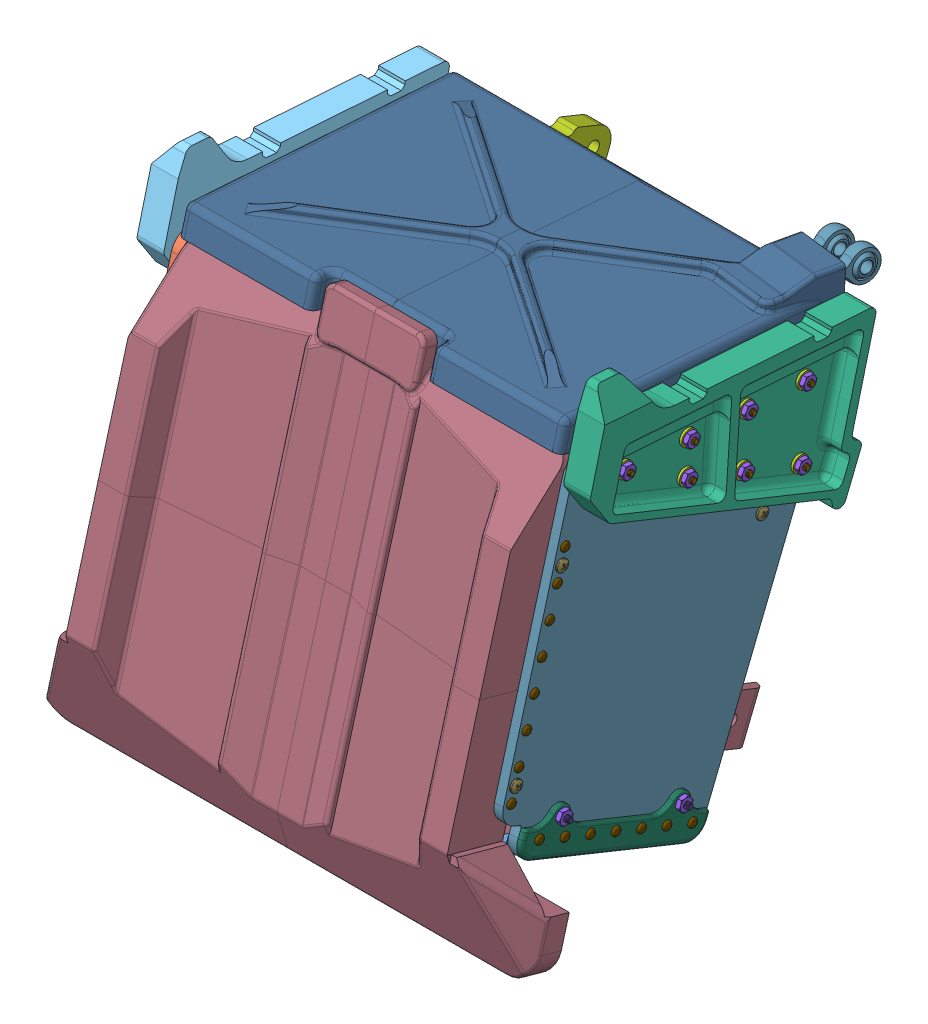
SolidWorks assembly Parachute Container, configuration Default. Lengths in mm. (continued)
Components (placement in the parent): (continued)
- 96765A145 - WASHER, .3125 X .750 X .05 THK, 18-8, BLK-3: 96765A145 - WASHER, .3125 X .750 X .05 THK, 18-8, BLK [96765A145] at (-114.4925 1025.2928 -878.0328) x (0.914596 0.374923 -0.151479) z (0.404368 -0.847999 0.342614) size (19.05 1.52 19.05)
- 91309A587 - HHCS, .3125 X 1.50, STEEL-3: 91309A587 - HHCS, .3125 X 1.50, STEEL [91309A587] at (-114.4925 1023.2114 -883.1845) x (-0.846075 -0.494248 0.199689) z (0 -0.374607 -0.927184) size (12.7 16.13 44.32)
- 92673A119 - NUT, .3125-18 X .50 HEX, 18-8-3: 92673A119 - NUT, .3125-18 X .50 HEX, 18-8 [92673A119] at (-114.4925 1036.6424 -849.9415) x (0.914596 0.374923 -0.151479) z (0 0.374607 0.927184) size (12.7 14.66 7.85)
- 96765A145 - WASHER, .3125 X .750 X .05 THK, 18-8, BLK-4: 96765A145 - WASHER, .3125 X .750 X .05 THK, 18-8, BLK [96765A145] at (-114.4925 861.3433 -811.7929) x (0.831512 0.515058 -0.208097) z (0.555507 -0.770964 0.31149) size (19.05 1.52 19.05)
- 91309A587 - HHCS, .3125 X 1.50, STEEL-4: 91309A587 - HHCS, .3125 X 1.50, STEEL [91309A587] at (-114.4925 859.2619 -816.9446) x (-0.741896 -0.621691 0.251179) z (0 -0.374607 -0.927184) size (12.7 16.13 44.32)
- 92673A119 - NUT, .3125-18 X .50 HEX, 18-8-4: 92673A119 - NUT, .3125-18 X .50 HEX, 18-8 [92673A119] at (-114.4925 872.6929 -783.7016) x (0.831512 0.515058 -0.208097) z (0 0.374607 0.927184) size (12.7 14.66 7.85)
- 4280_Black-1: 4280_Black [Default] at (91.075 1030.6212 -864.8445) x (0 0.927184 -0.374607) z (0 -0.374607 -0.927184) size (33.32 38.1 76.2)
- 4280_Black-2: 4280_Black [Default] at (91.075 866.6717 -798.6047) x (0 0.927184 -0.374607) z (0 -0.374607 -0.927184) size (33.32 38.1 76.2)
- 96765A145 - WASHER, .3125 X .750 X .05 THK, 18-8, BLK-1: 96765A145 - WASHER, .3125 X .750 X .05 THK, 18-8, BLK [96765A145] at (114.7605 1027.6715 -872.1452) x (1 0 0) z (0 -0.927184 0.374607) size (19.05 1.52 19.05)
- 91309A587 - HHCS, .3125 X 1.50, STEEL-1: 91309A587 - HHCS, .3125 X 1.50, STEEL [91309A587] at (114.7605 1025.5901 -877.2969) x (-0.989371 -0.134824 0.054473) z (0 -0.374607 -0.927184) size (12.7 16.13 44.32)
- 92673A119 - NUT, .3125-18 X .50 HEX, 18-8-1: 92673A119 - NUT, .3125-18 X .50 HEX, 18-8 [92673A119] at (114.7605 1036.6424 -849.9415) x (1 0 0) z (0 0.374607 0.927184) size (12.7 14.66 7.85)
- 96765A145 - WASHER, .3125 X .750 X .05 THK, 18-8, BLK-2: 96765A145 - WASHER, .3125 X .750 X .05 THK, 18-8, BLK [96765A145] at (114.7605 863.7221 -805.9053) x (0.976266 0.200807 -0.081131) z (0.216577 -0.905178 0.365716) size (19.05 1.52 19.05)
- 91309A587 - HHCS, .3125 X 1.50, STEEL-2: 91309A587 - HHCS, .3125 X 1.50, STEEL [91309A587] at (114.7605 861.6407 -811.057) x (-0.934396 -0.330297 0.133448) z (0 -0.374607 -0.927184) size (12.7 16.13 44.32)
- 92673A119 - NUT, .3125-18 X .50 HEX, 18-8-2: 92673A119 - NUT, .3125-18 X .50 HEX, 18-8 [92673A119] at (114.7605 872.6929 -783.7016) x (0.976266 0.200807 -0.081131) z (0 0.374607 0.927184) size (12.7 14.66 7.85)
- 60645K131 - ROD END, BALL JOINT, .3125-24 X 1.25 SHANK X .875 OAW, STEEL-1: 60645K131 - ROD END, BALL JOINT, .3125-24 X 1.25 SHANK X .875 OAW, STEEL [60645K131] at (108.1244 1115.527 -895.9272) x (0.040163 -0.996401 0.074652) z (0.990631 0.049467 0.127292) size (22.23 58.96 11.11)
- 60645K131 - ROD END, BALL JOINT, .3125-24 X 1.25 SHANK X .875 OAW, STEEL-2: 60645K131 - ROD END, BALL JOINT, .3125-24 X 1.25 SHANK X .875 OAW, STEEL [60645K131] at (129.7182 1116.6053 -893.1525) x (0.040163 -0.996401 0.074652) z (0.990631 0.049467 0.127292) size (22.23 58.96 11.11)
- 94846A510 - NUT, JAM, .3125-24 UNF X .500 HEX X .1875 THK, STL-1: 94846A510 - NUT, JAM, .3125-24 UNF X .500 HEX X .1875 THK, STL [94846A510] at (127.7497 1117.6435 -878.2364) x (0.991445 0.009063 0.130211) z (0 0.997587 -0.069434) size (12.7 5.58 14.66)
- 94846A510 - NUT, JAM, .3125-24 UNF X .500 HEX X .1875 THK, STL-2: 94846A510 - NUT, JAM, .3125-24 UNF X .500 HEX X .1875 THK, STL [94846A510] at (106.1559 1116.5652 -881.0111) x (-0.991445 -0.009063 -0.130211) z (0 -0.997587 0.069434) size (12.7 5.58 14.66)
Mates (geometry in assembly coordinates):
- Coincident591: coincident: plane of Outside Parachute Container Skin-1 through (142.1667 899.8015 -658.023) normal (0 0.374607 0.927184); line of Lower Parachute Container Skin Trim-1 through (142.1667 896.8577 -656.8337) axis (0 -0.927184 0.374607)
- Coincident592: coincident: plane of Outside Parachute Container Skin-1 through (142.1667 827.6721 -782.8478) normal (0 -0.927184 0.374607); line of Lower Parachute Container Skin Trim-1 through (142.1667 876.3918 -662.2623) axis (0 -0.374607 -0.927184)
- Coincident593: coincident anti-aligned: plane of Outside Parachute Container Skin-1 through (142.1667 927.3874 -569.9461) normal (1 0 0); plane of Lower Parachute Container Skin Trim-1 through (142.1667 844.2049 -775.8301) normal (-1 0 0)
- Concentric150: concentric anti-aligned: cylinder of LH Canopy Breaker-1 through (148.5167 1083.7351 -810.3922) axis (1 0 0) radius 2.4574; cylinder of 98023A113 - WASHER, #8, STEEL, ZINC-1 through (150.1677 1083.7351 -810.3922) axis (-1 0 0) radius 5.5563
- Coincident441: coincident anti-aligned: plane of LH Canopy Breaker-1 through (148.5167 927.3874 -569.9461) normal (1 0 0); plane of 98023A113 - WASHER, #8, STEEL, ZINC-1 through (148.5167 1083.7351 -810.3922) normal (-1 0 0)
- Concentric152: concentric aligned: circle of LH Canopy Breaker-1; cone of 90275A196 - FHS, 82 CSK, 8-32 X .625, STEEL, ZINC-1 through (139.2839 1083.7351 -810.3922) axis (1 0 0)
- Concentric151: concentric anti-aligned: circle of 90480A009 - NUT, 8-32, STEEL-1; circle of 98023A113 - WASHER, #8, STEEL, ZINC-1
- Coincident442: coincident anti-aligned: plane of 90480A009 - NUT, 8-32, STEEL-1 through (150.1677 1088.1574 -807.9726) normal (-1 0 0); plane of 98023A113 - WASHER, #8, STEEL, ZINC-1 through (150.1677 1083.7351 -810.3922) normal (1 0 0)
- Coincident617: coincident: plane of Outside Parachute Container Skin-1 through (135.8167 927.3874 -569.9461) normal (-1 0 0); plane of 90275A196 - FHS, 82 CSK, 8-32 X .625, STEEL, ZINC-1 through (139.2839 1082.4841 -808.7269) normal (-1 0 0)
- Coincident618: coincident aligned: cone of 90275A196 - FHS, 82 CSK, 8-32 X .625, STEEL, ZINC-1 through (139.2839 1083.7351 -810.3922) axis (1 0 0); cone of Outside Parachute Container Skin-1 through (135.8167 1083.7351 -810.3922) axis (1 0 0)
- Coincident419: coincident aligned: plane of Parachute Container Lid-1 through (-135.4148 1113.3918 -887.2968) normal (0 -0.069434 -0.997587); plane of Parachute Container Lid-2 through (-135.4148 1113.3918 -887.2968) normal (0 -0.069434 -0.997587)
- Coincident420: coincident anti-aligned: plane of Parachute Container Lid-1 through (0.268 1108.3189 -583.3878) normal (-1 0 0); plane of Parachute Container Lid-2 through (0.268 1108.3189 -583.3878) normal (1 0 0)
- Coincident421: coincident aligned: plane of Parachute Container Lid-1 through (-135.4148 1126.7365 -695.5689) normal (0 0.997587 -0.069434); plane of Parachute Container Lid-2 through (-135.4148 1126.7365 -695.5689) normal (0 0.997587 -0.069434)
- Concentric147: concentric anti-aligned: cone of Parachute Container Lid-1 through (110.5507 1087.7651 -860.052) axis (0 0.997252 -0.074087); cylinder of 93365A140 - INSERT, 8-32, BRASS, FOR PLASTICS-1 through (110.5507 1087.7651 -860.052) axis (0 -0.997252 0.074087) radius 2.8702
- Coincident438: coincident aligned: plane of Parachute Container Lid-1 through (135.9507 1108.3189 -583.3878) normal (0 -0.997252 0.074087); plane of 93365A140 - INSERT, 8-32, BRASS, FOR PLASTICS-1 through (110.5507 1087.7651 -860.052) normal (0 -0.997252 0.074087)
- Concentric145: concentric anti-aligned: circle of 93365A140 - INSERT, 8-32, BRASS, FOR PLASTICS-1; cylinder of 98023A113 - WASHER, #8, STEEL, ZINC-2 through (110.5507 1075.1 -859.111) axis (0 -0.997252 0.074087) radius 5.5563
- Concentric146: concentric aligned: cylinder of 98023A113 - WASHER, #8, STEEL, ZINC-2 through (110.5507 1073.4536 -858.9887) axis (0 0.997252 -0.074087) radius 2.3813; cylinder of 91249A197 - PHS, 8-32 x .750, 18-8, BLACK-OXIDE-1 through (110.5507 1092.4512 -860.4001) axis (0 0.997252 -0.074087) radius 4.0894
- Coincident437: coincident anti-aligned: plane of 98023A113 - WASHER, #8, STEEL, ZINC-2 through (110.5507 1073.4536 -858.9887) normal (0 -0.997252 0.074087); plane of 91249A197 - PHS, 8-32 x .750, 18-8, BLACK-OXIDE-1 through (110.5507 1073.4536 -858.9887) normal (0 0.997252 -0.074087)
- Coincident624: coincident anti-aligned: plane of Top Parachute Container Base-1 through (135.8167 1095.6538 -582.4469) normal (0 -0.997252 0.074087); plane of 98023A113 - WASHER, #8, STEEL, ZINC-2 through (110.5507 1075.1 -859.111) normal (0 0.997252 -0.074087)
- Coincident422: coincident aligned: plane of SJU-17 Headrest v2-1 through (0.134 1058.4473 -689.3362) normal (1 0 0); plane of SJU-17 Headrest v2-4 through (0.134 1058.4473 -689.3362) normal (1 0 0)
- Coincident423: coincident anti-aligned: plane of SJU-17 Headrest v2-1 through (25.6344 976.5404 -666.9102) normal (0 -0.964501 0.264079); plane of SJU-17 Headrest v2-4 through (25.6344 976.5404 -666.9102) normal (0 0.964501 -0.264079)
- Coincident424: coincident aligned: plane of SJU-17 Headrest v2-1 through (-39.7475 1284.261 -740.0242) normal (0.131243 0.261795 0.956158); plane of SJU-17 Headrest v2-4 through (-39.7475 1284.261 -740.0242) normal (0.131243 0.261795 0.956158)
- Coincident429: coincident anti-aligned: plane of SJU-17 Headrest v2-1 through (0.134 1058.4473 -689.3362) normal (1 0 0); plane of SJU-17 Headrest v2-2 through (0.134 1058.4473 -689.3362) normal (-1 0 0)
- Coincident626: coincident anti-aligned: plane of SJU-17 Headrest v2-1 through (-172.9084 529.51 -551.8216) normal (0 -0.264079 -0.964501); plane of Side Parachute Container Support-1 through (123.1167 1086.5973 -704.3515) normal (0 0.264079 0.964501)
- Distance52: distance = 16.3329 mm: line of ? through (-154.8427 837.9366 -655.5301) axis (1 0 0); plane of Lower Parachute Container Base-1 through (52.975 915.6122 -565.1886) normal (0 -0.927184 0.374607)
- Coincident636: coincident anti-aligned: plane of SJU-17 Headrest v2-1 through (-129.0297 1105.3946 -699.8136) normal (0 0.964501 -0.264079); plane of Parachute Container Lid-1 through (-135.4148 1107.9641 -690.429) normal (0 -0.964501 0.264079)
- Concentric143: concentric anti-aligned: circle of 93365A140 - INSERT, 8-32, BRASS, FOR PLASTICS-2; cylinder of 98023A113 - WASHER, #8, STEEL, ZINC-3 through (110.2446 1068.9512 -712.6875) axis (0 -0.264079 -0.964501) radius 5.5563
- Concentric144: concentric aligned: cylinder of 91249A197 - PHS, 8-32 x .750, 18-8, BLACK-OXIDE-2 through (110.2446 1073.5459 -695.9061) axis (0 0.264079 0.964501) radius 4.0894; cylinder of 98023A113 - WASHER, #8, STEEL, ZINC-3 through (110.2446 1068.5152 -714.2799) axis (0 0.264079 0.964501) radius 2.3813
- Coincident436: coincident anti-aligned: plane of 98023A113 - WASHER, #8, STEEL, ZINC-3 through (110.2446 1068.5152 -714.2799) normal (0 -0.264079 -0.964501); plane of 91249A197 - PHS, 8-32 x .750, 18-8, BLACK-OXIDE-2 through (110.2446 1068.5152 -714.2799) normal (0 0.264079 0.964501)
- Coincident623: coincident anti-aligned: plane of FWD Parachute Container Support-1 through (135.9507 900.9028 -666.676) normal (0 -0.264079 -0.964501); plane of 98023A113 - WASHER, #8, STEEL, ZINC-3 through (110.2446 1068.9512 -712.6875) normal (0 0.264079 0.964501)
- Concentric142: concentric anti-aligned: cone of SJU-17 Headrest v2-2 through (110.2446 1072.305 -700.4383) axis (0 0.264079 0.964501); cylinder of 93365A140 - INSERT, 8-32, BRASS, FOR PLASTICS-2 through (110.2446 1072.305 -700.4383) axis (0 -0.264079 -0.964501) radius 2.8702
- Coincident434: coincident aligned: plane of SJU-17 Headrest v2-2 through (-172.9084 529.51 -551.8216) normal (0 -0.264079 -0.964501); plane of 93365A140 - INSERT, 8-32, BRASS, FOR PLASTICS-2 through (110.2446 1072.305 -700.4383) normal (0 -0.264079 -0.964501)
- Coincident428: coincident anti-aligned: plane of SJU-17 Headrest v2-3 through (25.6344 976.5404 -666.9102) normal (0 0.964501 -0.264079); plane of SJU-17 Headrest v2-2 through (25.6344 976.5404 -666.9102) normal (0 -0.964501 0.264079)
- Coincident430: coincident aligned: plane of SJU-17 Headrest v2-3 through (40.0155 1284.261 -740.0242) normal (-0.131243 0.261795 0.956158); plane of SJU-17 Headrest v2-2 through (40.0155 1284.261 -740.0242) normal (-0.131243 0.261795 0.956158)
- Coincident425: coincident anti-aligned: plane of SJU-17 Headrest v2-4 through (0.134 1058.4473 -689.3362) normal (1 0 0); plane of SJU-17 Headrest v2-3 through (0.134 1058.4473 -689.3362) normal (-1 0 0)
- Coincident426: coincident aligned: plane of SJU-17 Headrest v2-4 through (25.6344 828.2767 -626.3157) normal (0 -0.964501 0.264079); plane of SJU-17 Headrest v2-3 through (25.6344 828.2767 -626.3157) normal (0 -0.964501 0.264079)
- Coincident427: coincident aligned: plane of SJU-17 Headrest v2-4 through (18.1951 1283.2496 -743.7181) normal (0 0.264079 0.964501); plane of SJU-17 Headrest v2-3 through (18.1951 1283.2496 -743.7181) normal (0 0.264079 0.964501)
- Width1: width anti-aligned: plane of Lower Parachute Container Base-1 through (-135.5488 839.4474 -787.6053) normal (-1 0 0); plane of FWD Parachute Container Support-1 through (135.8167 839.4474 -787.6053) normal (1 0 0); plane of Lower Parachute Container Base-1 through (123.2507 890.5693 -663.8467) normal (1 0 0); plane of FWD Parachute Container Support-1 through (-122.9828 890.5693 -663.8467) normal (-1 0 0)
- Concentric291: concentric anti-aligned: cylinder of Outside Parachute Container Skin-1 through (142.1667 1007.3681 -828.0549) axis (1 0 0) radius 2.4574; cylinder of 91249A197 - PHS, 8-32 x .750, 18-8, BLACK-OXIDE-3 through (123.1167 1007.3681 -828.0549) axis (-1 0 0) radius 4.0894
- Coincident622: coincident anti-aligned: plane of Outside Parachute Container Skin-1 through (142.1667 927.3874 -569.9461) normal (1 0 0); plane of 91249A197 - PHS, 8-32 x .750, 18-8, BLACK-OXIDE-3 through (142.1667 1007.3681 -828.0549) normal (-1 0 0)
- Concentric298: concentric anti-aligned: cylinder of Side Parachute Container Support-1 through (135.8167 1007.3681 -828.0549) axis (1 0 0) radius 2.9766; cone of 92105A660 - INSERT, 8-32, SELF TAPPING, FOR SOFTWOOD-1 through (135.8167 1007.3681 -828.0549) axis (-1 0 0)
- Coincident632: coincident aligned: plane of Side Parachute Container Support-1 through (135.8167 927.3874 -569.9461) normal (1 0 0); plane of 92105A660 - INSERT, 8-32, SELF TAPPING, FOR SOFTWOOD-1 through (135.8167 1007.3681 -828.0549) normal (1 0 0)
- Concentric287: concentric anti-aligned: cylinder of Lower Parachute Container Skin Trim-1 through (145.3417 860.255 -768.6173) axis (1 0 0) radius 2.4574; circle of 90480A009 - NUT, 8-32, STEEL-2
- Coincident616: coincident anti-aligned: plane of Lower Parachute Container Skin Trim-1 through (145.3417 844.2049 -775.8301) normal (1 0 0); plane of 90480A009 - NUT, 8-32, STEEL-2 through (145.3417 856.3442 -771.7981) normal (-1 0 0)
- Concentric296: concentric aligned: cylinder of Side Parachute Container Support-1 through (135.8167 860.255 -768.6173) axis (1 0 0) radius 2.9766; cone of 92105A660 - INSERT, 8-32, SELF TAPPING, FOR SOFTWOOD-2 through (123.1167 860.255 -768.6173) axis (1 0 0)
- Coincident630: coincident aligned: plane of Side Parachute Container Support-1 through (123.1167 927.3874 -569.9461) normal (-1 0 0); plane of 92105A660 - INSERT, 8-32, SELF TAPPING, FOR SOFTWOOD-2 through (123.1167 860.255 -768.6173) normal (-1 0 0)
- Concentric275: concentric anti-aligned: cylinder of 90272A201 - PHS, 8-32 x 1.250, STEEL, ZINC-1 through (151.6917 860.255 -768.6173) axis (1 0 0) radius 4.0894; circle of 90480A009 - NUT, 8-32, STEEL-3
- Coincident604: coincident anti-aligned: plane of 90272A201 - PHS, 8-32 x 1.250, STEEL, ZINC-1 through (119.9417 860.255 -768.6173) normal (1 0 0); plane of 90480A009 - NUT, 8-32, STEEL-3 through (119.9417 856.3442 -771.7981) normal (-1 0 0)
- Concentric297: concentric anti-aligned: cylinder of Side Parachute Container Support-1 through (135.8167 860.255 -768.6173) axis (1 0 0) radius 2.9766; circle of 90480A009 - NUT, 8-32, STEEL-3
- Coincident631: coincident anti-aligned: plane of Side Parachute Container Support-1 through (123.1167 927.3874 -569.9461) normal (-1 0 0); plane of 90480A009 - NUT, 8-32, STEEL-3 through (123.1167 856.3442 -771.7981) normal (1 0 0)
- Concentric274: concentric anti-aligned: circle of 90480A009 - NUT, 8-32, STEEL-4; cylinder of 90272A201 - PHS, 8-32 x 1.250, STEEL, ZINC-2 through (151.6917 894.7022 -683.3576) axis (1 0 0) radius 4.0894
- Coincident603: coincident anti-aligned: plane of 90480A009 - NUT, 8-32, STEEL-4 through (119.9417 890.3366 -685.8781) normal (-1 0 0); plane of 90272A201 - PHS, 8-32 x 1.250, STEEL, ZINC-2 through (119.9417 894.7022 -683.3576) normal (1 0 0)
- Concentric295: concentric anti-aligned: cylinder of Side Parachute Container Support-1 through (135.8167 894.7022 -683.3576) axis (1 0 0) radius 2.9766; circle of 90480A009 - NUT, 8-32, STEEL-4
- Coincident629: coincident anti-aligned: plane of Side Parachute Container Support-1 through (123.1167 927.3874 -569.9461) normal (-1 0 0); plane of 90480A009 - NUT, 8-32, STEEL-4 through (123.1167 890.3366 -685.8781) normal (1 0 0)
- Concentric294: concentric aligned: cylinder of Side Parachute Container Support-1 through (135.8167 894.7022 -683.3576) axis (1 0 0) radius 2.9766; cone of 92105A660 - INSERT, 8-32, SELF TAPPING, FOR SOFTWOOD-3 through (123.1167 894.7022 -683.3576) axis (1 0 0)
- Coincident628: coincident aligned: plane of Side Parachute Container Support-1 through (123.1167 927.3874 -569.9461) normal (-1 0 0); plane of 92105A660 - INSERT, 8-32, SELF TAPPING, FOR SOFTWOOD-3 through (123.1167 894.7022 -683.3576) normal (-1 0 0)
- Concentric286: concentric anti-aligned: circle of Lower Parachute Container Skin Trim-1; circle of 90480A009 - NUT, 8-32, STEEL-5
- Parallel31: parallel anti-aligned: plane of Lower Parachute Container Skin Trim-1 through (145.3417 844.2049 -775.8301) normal (1 0 0); plane of 90480A009 - NUT, 8-32, STEEL-5 through (145.3417 890.3366 -685.8781) normal (-1 0 0)
- Coincident615: coincident anti-aligned: plane of Lower Parachute Container Skin Trim-1 through (145.3417 844.2049 -775.8301) normal (1 0 0); plane of 90480A009 - NUT, 8-32, STEEL-5 through (145.3417 890.3366 -685.8781) normal (-1 0 0)
- Concentric290: concentric anti-aligned: cylinder of Outside Parachute Container Skin-1 through (142.1667 926.9171 -652.9942) axis (1 0 0) radius 2.4574; cylinder of 91249A197 - PHS, 8-32 x .750, 18-8, BLACK-OXIDE-4 through (123.1167 926.9171 -652.9942) axis (-1 0 0) radius 4.0894
- Coincident621: coincident anti-aligned: plane of Outside Parachute Container Skin-1 through (142.1667 927.3874 -569.9461) normal (1 0 0); plane of 91249A197 - PHS, 8-32 x .750, 18-8, BLACK-OXIDE-4 through (142.1667 926.9171 -652.9942) normal (-1 0 0)
- Concentric303: concentric anti-aligned: cone of SJU-17 Headrest v2-3 through (135.674 926.9158 -652.9941) axis (-1 -0.000201 0.000005); cylinder of 93365A140 - INSERT, 8-32, BRASS, FOR PLASTICS-3 through (135.674 926.9158 -652.9941) axis (1 0.000201 -0.000005) radius 2.8702
- Coincident639: coincident aligned: plane of SJU-17 Headrest v2-3 through (135.6382 1103.4543 -727.802) normal (1 0.000201 -0.000005); plane of 93365A140 - INSERT, 8-32, BRASS, FOR PLASTICS-3 through (135.674 926.9158 -652.9941) normal (1 0.000201 -0.000005)
- Concentric289: concentric anti-aligned: cylinder of Outside Parachute Container Skin-1 through (142.1667 1046.3464 -685.6938) axis (1 0 0) radius 2.4574; cylinder of 91249A197 - PHS, 8-32 x .750, 18-8, BLACK-OXIDE-5 through (123.1167 1046.3464 -685.6938) axis (-1 0 0) radius 4.0894
- Coincident620: coincident anti-aligned: plane of Outside Parachute Container Skin-1 through (142.1667 927.3874 -569.9461) normal (1 0 0); plane of 91249A197 - PHS, 8-32 x .750, 18-8, BLACK-OXIDE-5 through (142.1667 1046.3464 -685.6938) normal (-1 0 0)
- Concentric302: concentric anti-aligned: cone of SJU-17 Headrest v2-2 through (135.6498 1046.3451 -685.6937) axis (-1 -0.000201 0.000005); cylinder of 93365A140 - INSERT, 8-32, BRASS, FOR PLASTICS-4 through (135.6498 1046.3451 -685.6937) axis (1 0.000201 -0.000005) radius 2.8702
- Coincident638: coincident aligned: plane of SJU-17 Headrest v2-2 through (135.6382 1103.4543 -727.802) normal (1 0.000201 -0.000005); plane of 93365A140 - INSERT, 8-32, BRASS, FOR PLASTICS-4 through (135.6498 1046.3451 -685.6937) normal (1 0.000201 -0.000005)
- Concentric285: concentric anti-aligned: cylinder of Lower Parachute Container Skin Trim-1 through (145.3417 888.1671 -667.0198) axis (1 0 0) radius 1.5875; cylinder of 91654A144 - SCREW NAIL, DOMED, .14 X .25 SHANK X .25 HD DIA, 18-8-1 through (138.9917 888.1671 -667.0198) axis (-1 0 0) radius 1.778
- Coincident614: coincident anti-aligned: plane of Lower Parachute Container Skin Trim-1 through (145.3417 844.2049 -775.8301) normal (1 0 0); plane of 91654A144 - SCREW NAIL, DOMED, .14 X .25 SHANK X .25 HD DIA, 18-8-1 through (145.3417 889.2158 -668.4556) normal (-1 0 0)
- Concentric288: concentric anti-aligned: cylinder of Outside Parachute Container Skin-1 through (142.1667 1056.2989 -688.4187) axis (1 0 0) radius 1.5875; cylinder of 91654A144 - SCREW NAIL, DOMED, .14 X .25 SHANK X .25 HD DIA, 18-8-2 through (135.8167 1056.2989 -688.4187) axis (-1 0 0) radius 1.778
- Coincident619: coincident anti-aligned: plane of Outside Parachute Container Skin-1 through (142.1667 927.3874 -569.9461) normal (1 0 0); plane of 91654A144 - SCREW NAIL, DOMED, .14 X .25 SHANK X .25 HD DIA, 18-8-2 through (142.1667 1057.1067 -690.0027) normal (-1 0 0)
- Concentric292: concentric aligned: cone of Top Parachute Container Base-1 through (129.4667 1096.2173 -746.2814) axis (0 -0.997252 0.074087); cone of 90252A11X - FHS, 82 DEG, #8, BLK, STEEL, FOR MDF-1 through (129.4667 1091.9806 -745.9667) axis (0 -0.997252 0.074087)
- Coincident625: coincident aligned: cone of Top Parachute Container Base-1 through (129.4667 1096.2173 -746.2814) axis (0 -0.997252 0.074087); cone of 90252A11X - FHS, 82 DEG, #8, BLK, STEEL, FOR MDF-1 through (129.4667 1091.9806 -745.9667) axis (0 -0.997252 0.074087)
- Concentric293: concentric aligned: cone of Side Parachute Container Support-1 through (135.8167 1065.2704 -707.1666) axis (-1 0 0); cone of 90252A11X - FHS, 82 DEG, #8, BLK, STEEL, FOR MDF-2 through (131.5683 1065.2704 -707.1666) axis (-1 0 0)
- Coincident627: coincident aligned: cone of Side Parachute Container Support-1 through (135.8167 1065.2704 -707.1666) axis (-1 0 0); cone of 90252A11X - FHS, 82 DEG, #8, BLK, STEEL, FOR MDF-2 through (131.5683 1065.2704 -707.1666) axis (-1 0 0)
- Concentric299: concentric aligned: cone of Aft Parachute Container Support-1 through (129.4667 1050.1949 -872.7529) axis (0 0.374607 0.927184); cone of 90252A11X - FHS, 82 DEG, #8, BLK, STEEL, FOR MDF-3 through (129.4667 1051.7864 -868.8138) axis (0 0.374607 0.927184)
- Coincident633: coincident aligned: cone of Aft Parachute Container Support-1 through (129.4667 1050.1949 -872.7529) axis (0 0.374607 0.927184); cone of 90252A11X - FHS, 82 DEG, #8, BLK, STEEL, FOR MDF-3 through (129.4667 1051.7864 -868.8138) axis (0 0.374607 0.927184)
- Concentric301: concentric aligned: cone of Lower Parachute Container Base-1 through (129.4667 869.2556 -679.9252) axis (0 0.927184 -0.374607); cone of 90252A11X - FHS, 82 DEG, #8, BLK, STEEL, FOR MDF-4 through (129.4667 873.1946 -681.5166) axis (0 0.927184 -0.374607)
- Coincident635: coincident aligned: cone of Lower Parachute Container Base-1 through (129.4667 869.2556 -679.9252) axis (0 0.927184 -0.374607); cone of 90252A11X - FHS, 82 DEG, #8, BLK, STEEL, FOR MDF-4 through (129.4667 873.1946 -681.5166) axis (0 0.927184 -0.374607)
- Coincident690: coincident anti-aligned: plane of Aft Parachute Container Support-1 through (135.8167 1339.1648 -989.5042) normal (0 -0.374607 -0.927184); plane of RH Parachute Container Mount-1/PCM Parachute Container Interface Plate-1 through (53.243 839.4474 -787.6053) normal (0 0.374607 0.927184)
- Coincident723: coincident anti-aligned: plane of Aft Parachute Container Support-1 through (135.8167 1339.1648 -989.5042) normal (0 -0.374607 -0.927184); plane of 4280_Black-1 through (91.075 1046.0703 -871.0864) normal (0 0.374607 0.927184)
- Distance62: distance = 25.4 mm aligned: plane of 4280_Black-1 through (91.075 1019.904 -935.8502) normal (0 0.927184 -0.374607); plane of Aft Parachute Container Support-1 through (72.025 1069.6208 -880.6014) normal (0 0.927184 -0.374607)
- Coincident730: coincident anti-aligned: plane of 4280_Black-1 through (122.825 1043.6915 -876.974) normal (0 -0.374607 -0.927184); plane of 96765A145 - WASHER, .3125 X .750 X .05 THK, 18-8, BLK-1 through (114.7605 1028.2424 -870.7322) normal (0 0.374607 0.927184)
- Distance63: distance = 25.4 mm aligned: plane of 4280_Black-2 through (91.075 825.0563 -857.1266) normal (0 -0.927184 0.374607); plane of Lower Parachute Container Base-1 through (52.975 915.6122 -565.1886) normal (0 -0.927184 0.374607)
- Coincident724: coincident anti-aligned: plane of Aft Parachute Container Support-1 through (135.8167 1339.1648 -989.5042) normal (0 -0.374607 -0.927184); plane of 4280_Black-2 through (91.075 882.1208 -804.8465) normal (0 0.374607 0.927184)
- Concentric359: concentric aligned: cylinder of Aft Parachute Container Support-1 through (114.7605 1030.6212 -864.8445) axis (0 -0.374607 -0.927184) radius 4.365; cylinder of 96765A145 - WASHER, .3125 X .750 X .05 THK, 18-8, BLK-1 through (114.7605 1028.2424 -870.7322) axis (0 -0.374607 -0.927184) radius 9.525
- Coincident731: coincident anti-aligned: plane of 96765A145 - WASHER, .3125 X .750 X .05 THK, 18-8, BLK-1 through (114.7605 1027.6715 -872.1452) normal (0 -0.374607 -0.927184); plane of 91309A587 - HHCS, .3125 X 1.50, STEEL-1 through (114.7605 1027.6715 -872.1452) normal (0 0.374607 0.927184)
- Concentric362: concentric anti-aligned: cylinder of Aft Parachute Container Support-1 through (114.7605 1030.6212 -864.8445) axis (0 -0.374607 -0.927184) radius 4.365; circle of 91309A587 - HHCS, .3125 X 1.50, STEEL-1
- Coincident732: coincident anti-aligned: plane of Aft Parachute Container Support-1 through (135.8167 1343.9223 -977.729) normal (0 0.374607 0.927184); plane of 92673A119 - NUT, .3125-18 X .50 HEX, 18-8-1 through (108.4105 1038.7779 -854.4427) normal (0 -0.374607 -0.927184)
- Concentric363: concentric anti-aligned: cylinder of Aft Parachute Container Support-1 through (114.7605 1030.6212 -864.8445) axis (0 -0.374607 -0.927184) radius 4.365; circle of 92673A119 - NUT, .3125-18 X .50 HEX, 18-8-1
- Distance64: distance = 0.2001 mm aligned: plane of RH Parachute Container Mount-1/PCM Parachute Container Interface Plate-1 through (-135.5488 1064.6778 -892.3017) normal (0 0.927184 -0.374607); plane of Aft Parachute Container Support-1 through (72.025 1069.6208 -880.6014) normal (0 0.927184 -0.374607)
- Coincident733: coincident aligned: plane of Aft Parachute Container Support-1 through (-135.5488 1339.1648 -989.5042) normal (-1 0 0); plane of RH Parachute Container Mount-1/PCM Parachute Container Interface Plate-1 through (-135.5488 1064.6778 -892.3017) normal (-1 0 0)
- Distance65: distance = 181.882 mm anti-aligned: plane of 4280_Black-1 through (91.075 1017.5253 -941.7378) normal (-1 0 0); plane of RH Parachute Container Mount-1/PCM Upper Rail Interface Plate-1 through (-90.807 298.8807 -343.1935) normal (1 0 0)
- Coincident734: coincident aligned: plane of 4280_Black-1 through (91.075 1017.5253 -941.7378) normal (-1 0 0); plane of 4280_Black-2 through (91.075 853.5758 -875.4979) normal (-1 0 0)
- Coincident735: coincident anti-aligned: plane of 96765A145 - WASHER, .3125 X .750 X .05 THK, 18-8, BLK-2 through (114.7605 863.7221 -805.9053) normal (0 -0.374607 -0.927184); plane of 91309A587 - HHCS, .3125 X 1.50, STEEL-2 through (114.7605 863.7221 -805.9053) normal (0 0.374607 0.927184)
- Coincident736: coincident anti-aligned: plane of 4280_Black-2 through (122.825 879.7421 -810.7341) normal (0 -0.374607 -0.927184); plane of 96765A145 - WASHER, .3125 X .750 X .05 THK, 18-8, BLK-2 through (114.7605 864.293 -804.4923) normal (0 0.374607 0.927184)
- Concentric364: concentric aligned: cylinder of Aft Parachute Container Support-1 through (114.7605 866.6717 -798.6047) axis (0 -0.374607 -0.927184) radius 4.365; cylinder of 96765A145 - WASHER, .3125 X .750 X .05 THK, 18-8, BLK-2 through (114.7605 864.293 -804.4923) axis (0 -0.374607 -0.927184) radius 9.525
- Concentric365: concentric anti-aligned: cylinder of Aft Parachute Container Support-1 through (114.7605 866.6717 -798.6047) axis (0 -0.374607 -0.927184) radius 4.365; circle of 91309A587 - HHCS, .3125 X 1.50, STEEL-2
- Concentric366: concentric anti-aligned: cylinder of Aft Parachute Container Support-1 through (114.7605 866.6717 -798.6047) axis (0 -0.374607 -0.927184) radius 4.365; circle of 92673A119 - NUT, .3125-18 X .50 HEX, 18-8-2
- Coincident737: coincident anti-aligned: plane of Aft Parachute Container Support-1 through (135.8167 1343.9223 -977.729) normal (0 0.374607 0.927184); plane of 92673A119 - NUT, .3125-18 X .50 HEX, 18-8-2 through (107.7672 873.4726 -787.655) normal (0 -0.374607 -0.927184)
- Coincident738: coincident anti-aligned: plane of 96765A145 - WASHER, .3125 X .750 X .05 THK, 18-8, BLK-3 through (-114.4925 1025.2928 -878.0328) normal (0 -0.374607 -0.927184); plane of 91309A587 - HHCS, .3125 X 1.50, STEEL-3 through (-114.4925 1025.2928 -878.0328) normal (0 0.374607 0.927184)
- Coincident739: coincident anti-aligned: plane of Aft Parachute Container Support-1 through (135.8167 1343.9223 -977.729) normal (0 0.374607 0.927184); plane of 92673A119 - NUT, .3125-18 X .50 HEX, 18-8-3 through (-121.7827 1036.1068 -853.3635) normal (0 -0.374607 -0.927184)
- Coincident740: coincident anti-aligned: plane of RH Parachute Container Mount-1/PCM Parachute Container Interface Plate-1 through (53.243 834.6899 -799.3805) normal (0 -0.374607 -0.927184); plane of 96765A145 - WASHER, .3125 X .750 X .05 THK, 18-8, BLK-3 through (-114.4925 1025.8637 -876.6198) normal (0 0.374607 0.927184)
- Concentric367: concentric aligned: cylinder of Aft Parachute Container Support-1 through (-114.4925 1030.6212 -864.8445) axis (0 -0.374607 -0.927184) radius 4.365; cylinder of 96765A145 - WASHER, .3125 X .750 X .05 THK, 18-8, BLK-3 through (-114.4925 1025.8637 -876.6198) axis (0 -0.374607 -0.927184) radius 9.525
- Concentric368: concentric anti-aligned: cylinder of Aft Parachute Container Support-1 through (-114.4925 1030.6212 -864.8445) axis (0 -0.374607 -0.927184) radius 4.365; circle of 91309A587 - HHCS, .3125 X 1.50, STEEL-3
- Concentric369: concentric anti-aligned: cylinder of Aft Parachute Container Support-1 through (-114.4925 1030.6212 -864.8445) axis (0 -0.374607 -0.927184) radius 4.365; circle of 92673A119 - NUT, .3125-18 X .50 HEX, 18-8-3
- Coincident741: coincident anti-aligned: plane of 96765A145 - WASHER, .3125 X .750 X .05 THK, 18-8, BLK-4 through (-114.4925 861.3433 -811.7929) normal (0 -0.374607 -0.927184); plane of 91309A587 - HHCS, .3125 X 1.50, STEEL-4 through (-114.4925 861.3433 -811.7929) normal (0 0.374607 0.927184)
- Coincident742: coincident anti-aligned: plane of Aft Parachute Container Support-1 through (135.8167 1343.9223 -977.729) normal (0 0.374607 0.927184); plane of 92673A119 - NUT, .3125-18 X .50 HEX, 18-8-4 through (-121.8092 870.9851 -786.65) normal (0 -0.374607 -0.927184)
- Coincident743: coincident anti-aligned: plane of RH Parachute Container Mount-1/PCM Parachute Container Interface Plate-1 through (53.243 834.6899 -799.3805) normal (0 -0.374607 -0.927184); plane of 96765A145 - WASHER, .3125 X .750 X .05 THK, 18-8, BLK-4 through (-114.4925 861.9142 -810.3799) normal (0 0.374607 0.927184)
- Concentric370: concentric aligned: cylinder of Aft Parachute Container Support-1 through (-114.4925 866.6717 -798.6047) axis (0 -0.374607 -0.927184) radius 4.365; cylinder of 96765A145 - WASHER, .3125 X .750 X .05 THK, 18-8, BLK-4 through (-114.4925 861.9142 -810.3799) axis (0 -0.374607 -0.927184) radius 9.525
- Concentric371: concentric anti-aligned: cylinder of Aft Parachute Container Support-1 through (-114.4925 866.6717 -798.6047) axis (0 -0.374607 -0.927184) radius 4.365; circle of 91309A587 - HHCS, .3125 X 1.50, STEEL-4
- Concentric372: concentric anti-aligned: cylinder of Aft Parachute Container Support-1 through (-114.4925 866.6717 -798.6047) axis (0 -0.374607 -0.927184) radius 4.365; circle of 92673A119 - NUT, .3125-18 X .50 HEX, 18-8-4
- Concentric374: concentric: cylinder of Parachute Container Lid-1 through (108.1244 1115.527 -895.9272) axis (0.130526 -0.06884 -0.989052) radius 4.365; circle of 60645K141 - ROD END, BALL JOINT, .375-18 X 1.25 SHANK X 1.0 WIDTH, STL-1
- Parallel32: parallel: plane of Parachute Container Lid-1 through (131.1882 1110.2382 -841.153) normal (0.991445 0.009063 0.130211); plane of 60645K141 - ROD END, BALL JOINT, .375-18 X 1.25 SHANK X 1.0 WIDTH, STL-1 through (100.9226 1126.4813 -927.7759) normal (-0.996195 -0.006052 -0.086945)
- Concentric375: concentric: cylinder of Parachute Container Lid-1 through (129.7182 1116.6053 -893.1525) axis (0.130526 -0.06884 -0.989052) radius 4.365; circle of 60645K141 - ROD END, BALL JOINT, .375-18 X 1.25 SHANK X 1.0 WIDTH, STL-2
- Coincident748: coincident aligned: plane of Parachute Container Lid-1 through (137.8189 1106.7411 -891.3969) normal (0.130526 -0.06884 -0.989052); plane of 60645K141 - ROD END, BALL JOINT, .375-18 X 1.25 SHANK X 1.0 WIDTH, STL-1 through (102.8405 1115.9259 -896.5221) normal (0.087156 -0.06917 -0.99379)
- Coincident749: coincident aligned: plane of Parachute Container Lid-1 through (137.8189 1106.7411 -891.3969) normal (0.130526 -0.06884 -0.989052); plane of 60645K141 - ROD END, BALL JOINT, .375-18 X 1.25 SHANK X 1.0 WIDTH, STL-2 through (132.0839 1113.9698 -924.7039) normal (0.087156 -0.06917 -0.99379)
- Concentric376: concentric anti-aligned: cylinder of Parachute Container Lid-1 through (108.1244 1115.527 -895.9272) axis (0.130526 -0.06884 -0.989052) radius 4.365; circle of 60645K131 - ROD END, BALL JOINT, .3125-24 X 1.25 SHANK X .875 OAW, STEEL-1
- Coincident750: coincident aligned: plane of Parachute Container Lid-1 through (137.8189 1106.7411 -891.3969) normal (0.130526 -0.06884 -0.989052); plane of 60645K131 - ROD END, BALL JOINT, .3125-24 X 1.25 SHANK X .875 OAW, STEEL-1 through (108.1244 1115.527 -895.9272) normal (0.130526 -0.06884 -0.989052)
- Coincident751: coincident aligned: plane of Parachute Container Lid-1 through (137.8189 1106.7411 -891.3969) normal (0.130526 -0.06884 -0.989052); plane of 60645K131 - ROD END, BALL JOINT, .3125-24 X 1.25 SHANK X .875 OAW, STEEL-2 through (129.7182 1116.6053 -893.1525) normal (0.130526 -0.06884 -0.989052)
- Concentric377: concentric anti-aligned: cylinder of Parachute Container Lid-1 through (129.7182 1116.6053 -893.1525) axis (0.130526 -0.06884 -0.989052) radius 4.365; circle of 60645K131 - ROD END, BALL JOINT, .3125-24 X 1.25 SHANK X .875 OAW, STEEL-2
- Parallel36: parallel anti-aligned: plane of Parachute Container Lid-1 through (118.93 1116.0666 -894.5387) normal (-0.990631 -0.049467 -0.127292); plane of 60645K131 - ROD END, BALL JOINT, .3125-24 X 1.25 SHANK X .875 OAW, STEEL-1 through (108.1244 1115.527 -895.9272) normal (0.990631 0.049467 0.127292)
- Parallel37: parallel anti-aligned: plane of Parachute Container Lid-1 through (118.93 1116.0666 -894.5387) normal (-0.990631 -0.049467 -0.127292); plane of 60645K131 - ROD END, BALL JOINT, .3125-24 X 1.25 SHANK X .875 OAW, STEEL-2 through (129.7182 1116.6053 -893.1525) normal (0.990631 0.049467 0.127292)
- Concentric378: concentric anti-aligned: cylinder of Parachute Container Lid-1 through (129.7182 1116.6053 -893.1525) axis (0.130526 -0.06884 -0.989052) radius 4.365; circle of 94846A510 - NUT, JAM, .3125-24 UNF X .500 HEX X .1875 THK, STL-1
- Parallel38: parallel anti-aligned: plane of Parachute Container Lid-1 through (134.3227 1121.9157 -874.9376) normal (-0.991445 -0.009063 -0.130211); plane of 94846A510 - NUT, JAM, .3125-24 UNF X .500 HEX X .1875 THK, STL-1 through (134.3562 1121.1945 -880.0193) normal (0.991445 0.009063 0.130211)
- Coincident753: coincident anti-aligned: plane of Parachute Container Lid-1 through (174.1021 1088.1977 -872.4773) normal (-0.130526 0.06884 0.989052); plane of 94846A510 - NUT, JAM, .3125-24 UNF X .500 HEX X .1875 THK, STL-1 through (121.7649 1113.7647 -881.1638) normal (0.130526 -0.06884 -0.989052)
- Concentric379: concentric anti-aligned: cylinder of Parachute Container Lid-1 through (108.1244 1115.527 -895.9272) axis (0.130526 -0.06884 -0.989052) radius 4.365; circle of 94846A510 - NUT, JAM, .3125-24 UNF X .500 HEX X .1875 THK, STL-2
- Parallel39: parallel anti-aligned: plane of Parachute Container Lid-1 through (98.8784 1112.6647 -878.9714) normal (0.991445 0.009063 0.130211); plane of 94846A510 - NUT, JAM, .3125-24 UNF X .500 HEX X .1875 THK, STL-2 through (100.1711 1112.6864 -883.9385) normal (-0.991445 -0.009063 -0.130211)
- Coincident754: coincident anti-aligned: plane of Parachute Container Lid-1 through (174.1021 1088.1977 -872.4773) normal (-0.130526 0.06884 0.989052); plane of 94846A510 - NUT, JAM, .3125-24 UNF X .500 HEX X .1875 THK, STL-2 through (112.7624 1120.1162 -882.794) normal (0.130526 -0.06884 -0.989052)
